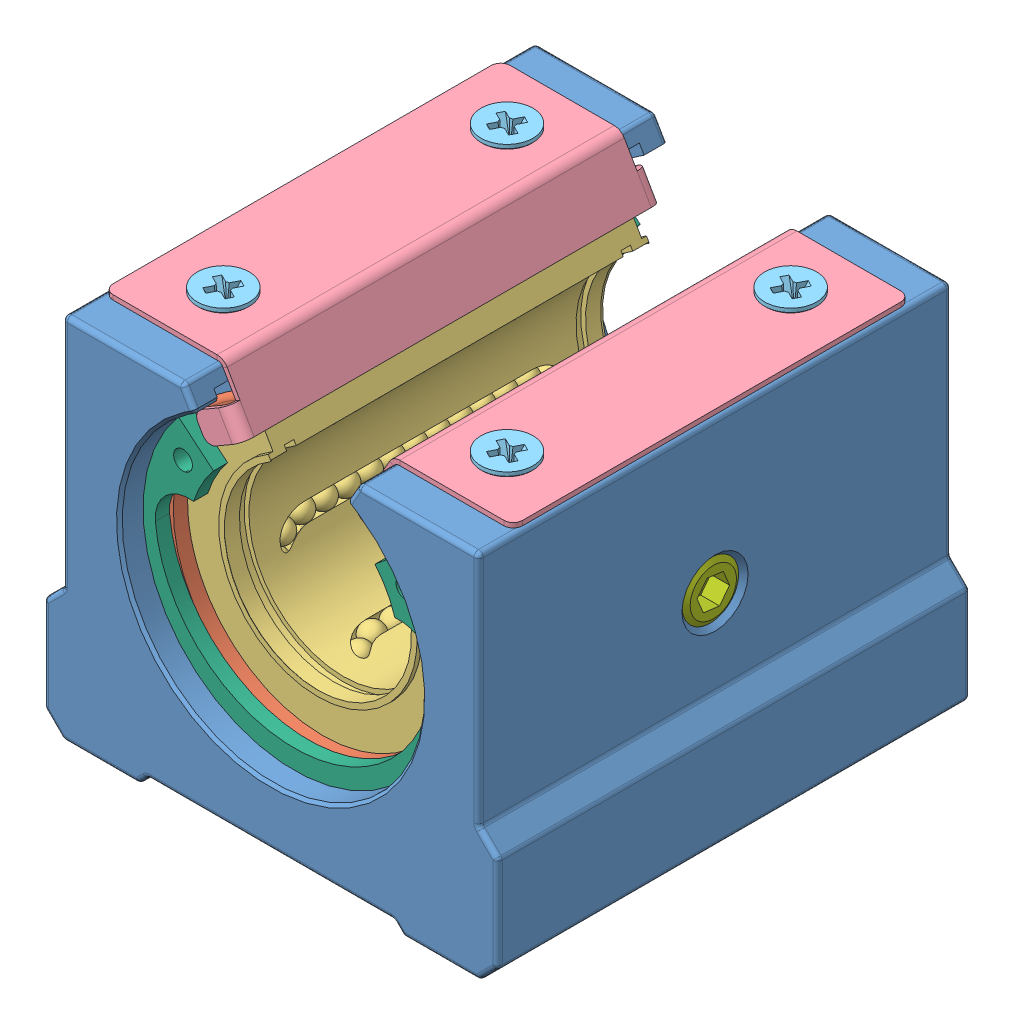
SolidWorks assembly SME20, configuration Default. Lengths in mm.
Overall size (48 42.63 50.13).
14 component instances, 7 part files, 16 mates.
Components (placement in the parent):
- SME20-1-1: SME20-1 [Default] at (-5.7284 29.1482 -16.78) size (48 39.1 50.13)
- LM20OP-2: LM20OP [Default] at (-3.2118 9.9406 8.4417) size (39.07 39.07 42.07)
  - LM20OP-1-2: LM20OP-1 [Default] at (-2.5166 3.2076 -21.2217) size (32 29.9 42.07)
  - LM20OP-2-2: LM20OP-2 [Default] at (4.6334 15.5917 -0.2217) x (0 0 -1) z (-0.5 -0.866025 0) size (40 28.6 28.6)
- SME20-2-3: SME20-2 [Default] at (6.4345 29.1482 5.6825) x (1 0 0) z (0 0 -1) size (15.92 7.34 44.47)
- SME20-2-4: SME20-2 [Default] at (-17.8913 29.1482 10.7574) x (-1 0 0) z (0 0 1) size (15.92 7.34 44.47)
- countersunk flat head cross recess screw_iso-2: countersunk flat head cross recess screw_iso [ISO 7046-1 - M3 x 4 - Z --- 4N] at (9.2716 30.1892 -6.78) x (0 -1 0) z (-0.452249 0 0.891892) size (4 5.5 5.5)
- countersunk flat head cross recess screw_iso-3: countersunk flat head cross recess screw_iso [ISO 7046-1 - M3 x 4 - Z --- 4N] at (9.2716 30.1892 23.22) x (0 -1 0) z (-0.452249 0 0.891892) size (4 5.5 5.5)
- countersunk flat head cross recess screw_iso-4: countersunk flat head cross recess screw_iso [ISO 7046-1 - M3 x 4 - Z --- 4N] at (-20.7284 30.1892 -6.78) x (0 -1 0) z (-0.452249 0 0.891892) size (4 5.5 5.5)
- countersunk flat head cross recess screw_iso-5: countersunk flat head cross recess screw_iso [ISO 7046-1 - M3 x 4 - Z --- 4N] at (-20.7284 30.1892 23.22) x (0 -1 0) z (-0.452249 0 0.891892) size (4 5.5 5.5)
- SME20-3-1: SME20-3 [Default] at (-5.7284 13.1482 29.22) x (-1 0 0) z (0 0 1) size (34 27.93 1.5)
- SME20-3-2: SME20-3 [Default] at (-5.7284 13.1482 -14.28) x (-0.999848 0.017452 0) z (0 0 1) size (34 27.93 1.5)
- socket set screw flat point_din-1: socket set screw flat point_din [DIN 913 - M4 x 4-N] at (-5.7284 -8.077 8.22) x (0 1 0) z (0 0 1) size (4 4 4)
- socket set screw flat point_din-2: socket set screw flat point_din [DIN 913 - M6 x 6-N] at (16.0917 13.1482 8.22) x (-1 0 0) z (0 -0.924225 -0.381849) size (6 6 6)
Mates (geometry in assembly coordinates):
- Concentric2: concentric aligned: cylinder of SME20-1-1 through (-5.7284 13.1482 33.22) axis (0 0 -1) radius 16; cylinder of LM20OP-2/LM20OP-1-2 through (-5.7284 13.1482 29.22) axis (0 0 -1) radius 16
- Coincident7: coincident anti-aligned: plane of SME20-1-1 through (3.5092 29.1482 33.22) normal (0 1 0); plane of SME20-2-3 through (15.9345 29.1482 -12.78) normal (0 -1 0)
- Coincident8: coincident anti-aligned: plane of SME20-1-1 through (2.2716 27.0046 33.22) normal (-0.866025 0.5 0); plane of SME20-2-3 through (9.944 40.2937 -12.78) normal (0.866025 -0.5 0)
- Coincident9: coincident aligned: plane of LM20OP-2/LM20OP-1-2 through (-5.7284 13.1482 29.22) normal (0 0 1); plane of SME20-2-3 through (-0.0655 29.6482 29.22) normal (0 0 1)
- Coincident10: coincident anti-aligned: plane of SME20-1-1 through (-14.966 29.1482 33.22) normal (0 1 0); plane of SME20-2-4 through (-27.3913 29.1482 29.22) normal (0 -1 0)
- Coincident11: coincident anti-aligned: plane of SME20-1-1 through (-13.7284 27.0046 33.22) normal (0.866025 0.5 0); plane of SME20-2-4 through (-21.4009 40.2937 29.22) normal (-0.866025 -0.5 0)
- Coincident12: coincident aligned: plane of LM20OP-2/LM20OP-1-2 through (-5.7284 13.1482 29.22) normal (0 0 1); plane of SME20-2-4 through (-11.3913 29.6482 29.22) normal (0 0 1)
- Concentric5: concentric aligned: cylinder of SME20-1-1 through (9.2716 24.1482 -6.78) axis (0 1 0) radius 2; cylinder of countersunk flat head cross recess screw_iso-2 through (9.2716 36.5392 -6.78) axis (0 1 0) radius 2.75
- Coincident13: coincident anti-aligned: plane of SME20-1-1 through (-5.7284 -2.8518 30.72) normal (0 0 -1); plane of SME20-3-1 through (-5.7284 13.1482 30.72) normal (0 0 1)
- Concentric6: concentric anti-aligned: cylinder of SME20-1-1 through (-5.7284 13.1482 33.22) axis (0 0 1) radius 17; cylinder of SME20-3-1 through (-5.7284 13.1482 30.72) axis (0 0 -1) radius 17
- Coincident15: coincident anti-aligned: plane of SME20-1-1 through (-5.7284 -2.8518 -14.28) normal (0 0 1); plane of SME20-3-2 through (-5.7284 13.1482 -14.28) normal (0 0 -1)
- Concentric7: concentric anti-aligned: cylinder of SME20-1-1 through (-5.7284 13.1482 33.22) axis (0 0 1) radius 17; cylinder of SME20-3-2 through (-5.7284 13.1482 -12.78) axis (0 0 -1) radius 17
- Concentric8: concentric aligned: cylinder of SME20-1-1 through (-5.7284 29.1492 8.22) axis (0 -1 0) radius 2; cylinder of socket set screw flat point_din-1 through (-5.7284 -20.777 8.22) axis (0 -1 0) radius 2
- Coincident16: coincident aligned: circle of SME20-1-1; circle of socket set screw flat point_din-1
- Concentric9: concentric aligned: cylinder of SME20-1-1 through (-29.7294 13.1482 8.22) axis (1 0 0) radius 3; cylinder of socket set screw flat point_din-2 through (28.7917 13.1482 8.22) axis (1 0 0) radius 3
- Coincident17: coincident aligned: circle of SME20-1-1; circle of socket set screw flat point_din-2
